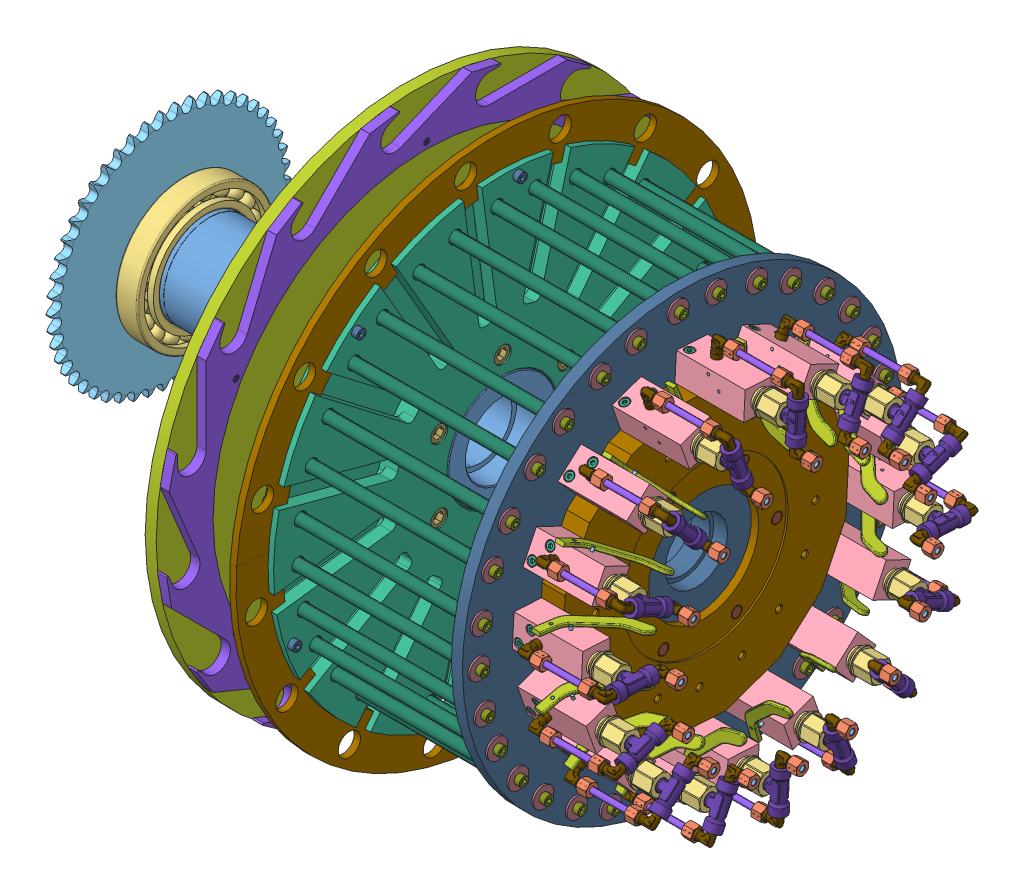
SolidWorks assembly assieme parte rotante, configuration Default. Lengths in mm. (continued)
Components (placement in the parent): (continued)
- AssiemeValvola-7: AssiemeValvola [Default] at (515.3257 -134.8578 488.6421) x (0 0.901303 -0.433189) z (0 -0.433189 -0.901303) size (90.26 138.63 38)
  - RaccordoT-1: RaccordoT [Default] at origin size (43 29.75 16.5)
  - Raccordo a L-1: Raccordo a L [Default] at (-30 0 0) x (0 -1 0) z (0 0 -1) size (28.34 25.51 14.01)
    - 1809_06_10_01-1: 1809_06_10_01 [Default] at origin size (22.49 23 10)
    - 1809_06_10_02-1: 1809_06_10_02 [Default] at origin size (6.5 8.5 8.5)
    - 1809_06_10_03-1: 1809_06_10_03 [Default] at origin size (11.02 15.01 14.01)
  - Raccordo a L-2: Raccordo a L [Default] at (30 0 0) x (0 1 0) z (0 0 -1) size (28.34 25.51 14.01)
    - 1809_06_10_01-1: 1809_06_10_01 [Default] at origin size (22.49 23 10)
    - 1809_06_10_02-1: 1809_06_10_02 [Default] at origin size (6.5 8.5 8.5)
    - 1809_06_10_03-1: 1809_06_10_03 [Default] at origin size (11.02 15.01 14.01)
  - TappoChiusura-1: TappoChiusura [Default] at (0 -32 0) x (0 -1 0) z (0 0 1) size (38.28 26.74 26.74)
  - CorpoValvola-1: CorpoValvola [Default] at (-15 -115.2824 0) size (30 75 34)
  - Raccordo a L-3: Raccordo a L [Default] at (-30 -88.2824 0) x (0 1 0) z (0 0 1) size (28.34 25.51 14.01)
    - 1809_06_10_01-1: 1809_06_10_01 [Default] at origin size (22.49 23 10)
    - 1809_06_10_02-1: 1809_06_10_02 [Default] at origin size (6.5 8.5 8.5)
    - 1809_06_10_03-1: 1809_06_10_03 [Default] at origin size (11.02 15.01 14.01)
  - Spina_3x38-1: Spina_3x38 [Default] at (0 -68.2824 -21) x (-1 0 0) z (0 0 1) size (3 3 38)
  - Spina_3x38-2: Spina_3x38 [Default] at (-10 -80.2824 -21) x (0.996193 0.087174 0) z (0 0 1) size (3 3 38)
  - M5 40mm-3: M5 40mm [ISO 4762 M5 x 40 - 40N] at (-14.6 -108.7824 9) size (45 8.5 8.5)
  - M5 40mm-2: M5 40mm [ISO 4762 M5 x 40 - 40N] at (-14.6 -96.7824 -9) size (45 8.5 8.5)
  - LevaValvola-1: LevaValvola [Default] at (-24.507 -86.571 -17) x (0.996193 0.087174 0) z (0 0 1) size (77.55 60.2 4)
  - Tubo-1: Tubo [Default] at (-30 -15.9665 0) x (1 0 0) z (0 -1 0) size (6 6 56.4)
- AssiemeValvola-8: AssiemeValvola [Default] at (515.3257 -95.0129 541.6718) x (0 0.666921 -0.745128) z (0 -0.745128 -0.666921) size (90.26 138.63 38)
  - RaccordoT-1: RaccordoT [Default] at origin size (43 29.75 16.5)
  - Raccordo a L-1: Raccordo a L [Default] at (-30 0 0) x (0 -1 0) z (0 0 -1) size (28.34 25.51 14.01)
    - 1809_06_10_01-1: 1809_06_10_01 [Default] at origin size (22.49 23 10)
    - 1809_06_10_02-1: 1809_06_10_02 [Default] at origin size (6.5 8.5 8.5)
    - 1809_06_10_03-1: 1809_06_10_03 [Default] at origin size (11.02 15.01 14.01)
  - Raccordo a L-2: Raccordo a L [Default] at (30 0 0) x (0 1 0) z (0 0 -1) size (28.34 25.51 14.01)
    - 1809_06_10_01-1: 1809_06_10_01 [Default] at origin size (22.49 23 10)
    - 1809_06_10_02-1: 1809_06_10_02 [Default] at origin size (6.5 8.5 8.5)
    - 1809_06_10_03-1: 1809_06_10_03 [Default] at origin size (11.02 15.01 14.01)
  - TappoChiusura-1: TappoChiusura [Default] at (0 -32 0) x (0 -1 0) z (0 0 1) size (38.28 26.74 26.74)
  - CorpoValvola-1: CorpoValvola [Default] at (-15 -115.2824 0) size (30 75 34)
  - Raccordo a L-3: Raccordo a L [Default] at (-30 -88.2824 0) x (0 1 0) z (0 0 1) size (28.34 25.51 14.01)
    - 1809_06_10_01-1: 1809_06_10_01 [Default] at origin size (22.49 23 10)
    - 1809_06_10_02-1: 1809_06_10_02 [Default] at origin size (6.5 8.5 8.5)
    - 1809_06_10_03-1: 1809_06_10_03 [Default] at origin size (11.02 15.01 14.01)
  - Spina_3x38-1: Spina_3x38 [Default] at (0 -68.2824 -21) x (-1 0 0) z (0 0 1) size (3 3 38)
  - Spina_3x38-2: Spina_3x38 [Default] at (-10 -80.2824 -21) x (0.996193 0.087174 0) z (0 0 1) size (3 3 38)
  - M5 40mm-3: M5 40mm [ISO 4762 M5 x 40 - 40N] at (-14.6 -108.7824 9) size (45 8.5 8.5)
  - M5 40mm-2: M5 40mm [ISO 4762 M5 x 40 - 40N] at (-14.6 -96.7824 -9) size (45 8.5 8.5)
  - LevaValvola-1: LevaValvola [Default] at (-24.507 -86.571 -17) x (0.996193 0.087174 0) z (0 0 1) size (77.55 60.2 4)
  - Tubo-1: Tubo [Default] at (-30 -15.9665 0) x (1 0 0) z (0 -1 0) size (6 6 56.4)
- AssiemeValvola-9: AssiemeValvola [Default] at (515.3257 -37.9074 575.4168) x (0 0.331007 -0.943628) z (0 -0.943628 -0.331007) size (90.26 138.63 38)
  - RaccordoT-1: RaccordoT [Default] at origin size (43 29.75 16.5)
  - Raccordo a L-1: Raccordo a L [Default] at (-30 0 0) x (0 -1 0) z (0 0 -1) size (28.34 25.51 14.01)
    - 1809_06_10_01-1: 1809_06_10_01 [Default] at origin size (22.49 23 10)
    - 1809_06_10_02-1: 1809_06_10_02 [Default] at origin size (6.5 8.5 8.5)
    - 1809_06_10_03-1: 1809_06_10_03 [Default] at origin size (11.02 15.01 14.01)
  - Raccordo a L-2: Raccordo a L [Default] at (30 0 0) x (0 1 0) z (0 0 -1) size (28.34 25.51 14.01)
    - 1809_06_10_01-1: 1809_06_10_01 [Default] at origin size (22.49 23 10)
    - 1809_06_10_02-1: 1809_06_10_02 [Default] at origin size (6.5 8.5 8.5)
    - 1809_06_10_03-1: 1809_06_10_03 [Default] at origin size (11.02 15.01 14.01)
  - TappoChiusura-1: TappoChiusura [Default] at (0 -32 0) x (0 -1 0) z (0 0 1) size (38.28 26.74 26.74)
  - CorpoValvola-1: CorpoValvola [Default] at (-15 -115.2824 0) size (30 75 34)
  - Raccordo a L-3: Raccordo a L [Default] at (-30 -88.2824 0) x (0 1 0) z (0 0 1) size (28.34 25.51 14.01)
    - 1809_06_10_01-1: 1809_06_10_01 [Default] at origin size (22.49 23 10)
    - 1809_06_10_02-1: 1809_06_10_02 [Default] at origin size (6.5 8.5 8.5)
    - 1809_06_10_03-1: 1809_06_10_03 [Default] at origin size (11.02 15.01 14.01)
  - Spina_3x38-1: Spina_3x38 [Default] at (0 -68.2824 -21) x (-1 0 0) z (0 0 1) size (3 3 38)
  - Spina_3x38-2: Spina_3x38 [Default] at (-10 -80.2824 -21) x (0.996193 0.087174 0) z (0 0 1) size (3 3 38)
  - M5 40mm-3: M5 40mm [ISO 4762 M5 x 40 - 40N] at (-14.6 -108.7824 9) size (45 8.5 8.5)
  - M5 40mm-2: M5 40mm [ISO 4762 M5 x 40 - 40N] at (-14.6 -96.7824 -9) size (45 8.5 8.5)
  - LevaValvola-1: LevaValvola [Default] at (-24.507 -86.571 -17) x (0.996193 0.087174 0) z (0 0 1) size (77.55 60.2 4)
  - Tubo-1: Tubo [Default] at (-30 -15.9665 0) x (1 0 0) z (0 -1 0) size (6 6 56.4)
- AssiemeValvola-10: AssiemeValvola [Default] at (515.3257 27.7648 584.7399) x (0 -0.055301 -0.99847) z (0 -0.99847 0.055301) size (90.26 138.63 38)
  - RaccordoT-1: RaccordoT [Default] at origin size (43 29.75 16.5)
  - Raccordo a L-1: Raccordo a L [Default] at (-30 0 0) x (0 -1 0) z (0 0 -1) size (28.34 25.51 14.01)
    - 1809_06_10_01-1: 1809_06_10_01 [Default] at origin size (22.49 23 10)
    - 1809_06_10_02-1: 1809_06_10_02 [Default] at origin size (6.5 8.5 8.5)
    - 1809_06_10_03-1: 1809_06_10_03 [Default] at origin size (11.02 15.01 14.01)
  - Raccordo a L-2: Raccordo a L [Default] at (30 0 0) x (0 1 0) z (0 0 -1) size (28.34 25.51 14.01)
    - 1809_06_10_01-1: 1809_06_10_01 [Default] at origin size (22.49 23 10)
    - 1809_06_10_02-1: 1809_06_10_02 [Default] at origin size (6.5 8.5 8.5)
    - 1809_06_10_03-1: 1809_06_10_03 [Default] at origin size (11.02 15.01 14.01)
  - TappoChiusura-1: TappoChiusura [Default] at (0 -32 0) x (0 -1 0) z (0 0 1) size (38.28 26.74 26.74)
  - CorpoValvola-1: CorpoValvola [Default] at (-15 -115.2824 0) size (30 75 34)
  - Raccordo a L-3: Raccordo a L [Default] at (-30 -88.2824 0) x (0 1 0) z (0 0 1) size (28.34 25.51 14.01)
    - 1809_06_10_01-1: 1809_06_10_01 [Default] at origin size (22.49 23 10)
    - 1809_06_10_02-1: 1809_06_10_02 [Default] at origin size (6.5 8.5 8.5)
    - 1809_06_10_03-1: 1809_06_10_03 [Default] at origin size (11.02 15.01 14.01)
  - Spina_3x38-1: Spina_3x38 [Default] at (0 -68.2824 -21) x (-1 0 0) z (0 0 1) size (3 3 38)
  - Spina_3x38-2: Spina_3x38 [Default] at (-10 -80.2824 -21) x (0.996193 0.087174 0) z (0 0 1) size (3 3 38)
  - M5 40mm-3: M5 40mm [ISO 4762 M5 x 40 - 40N] at (-14.6 -108.7824 9) size (45 8.5 8.5)
  - M5 40mm-2: M5 40mm [ISO 4762 M5 x 40 - 40N] at (-14.6 -96.7824 -9) size (45 8.5 8.5)
  - LevaValvola-1: LevaValvola [Default] at (-24.507 -86.571 -17) x (0.996193 0.087174 0) z (0 0 1) size (77.55 60.2 4)
  - Tubo-1: Tubo [Default] at (-30 -15.9665 0) x (1 0 0) z (0 -1 0) size (6 6 56.4)
- AssiemeValvola-11: AssiemeValvola [Default] at (515.3257 92.0058 568.2215) x (0 -0.433189 -0.901303) z (0 -0.901303 0.433189) size (90.26 138.63 38)
  - RaccordoT-1: RaccordoT [Default] at origin size (43 29.75 16.5)
  - Raccordo a L-1: Raccordo a L [Default] at (-30 0 0) x (0 -1 0) z (0 0 -1) size (28.34 25.51 14.01)
    - 1809_06_10_01-1: 1809_06_10_01 [Default] at origin size (22.49 23 10)
    - 1809_06_10_02-1: 1809_06_10_02 [Default] at origin size (6.5 8.5 8.5)
    - 1809_06_10_03-1: 1809_06_10_03 [Default] at origin size (11.02 15.01 14.01)
  - Raccordo a L-2: Raccordo a L [Default] at (30 0 0) x (0 1 0) z (0 0 -1) size (28.34 25.51 14.01)
    - 1809_06_10_01-1: 1809_06_10_01 [Default] at origin size (22.49 23 10)
    - 1809_06_10_02-1: 1809_06_10_02 [Default] at origin size (6.5 8.5 8.5)
    - 1809_06_10_03-1: 1809_06_10_03 [Default] at origin size (11.02 15.01 14.01)
  - TappoChiusura-1: TappoChiusura [Default] at (0 -32 0) x (0 -1 0) z (0 0 1) size (38.28 26.74 26.74)
  - CorpoValvola-1: CorpoValvola [Default] at (-15 -115.2824 0) size (30 75 34)
  - Raccordo a L-3: Raccordo a L [Default] at (-30 -88.2824 0) x (0 1 0) z (0 0 1) size (28.34 25.51 14.01)
    - 1809_06_10_01-1: 1809_06_10_01 [Default] at origin size (22.49 23 10)
    - 1809_06_10_02-1: 1809_06_10_02 [Default] at origin size (6.5 8.5 8.5)
    - 1809_06_10_03-1: 1809_06_10_03 [Default] at origin size (11.02 15.01 14.01)
  - Spina_3x38-1: Spina_3x38 [Default] at (0 -68.2824 -21) x (-1 0 0) z (0 0 1) size (3 3 38)
  - Spina_3x38-2: Spina_3x38 [Default] at (-10 -80.2824 -21) x (0.996193 0.087174 0) z (0 0 1) size (3 3 38)
  - M5 40mm-3: M5 40mm [ISO 4762 M5 x 40 - 40N] at (-14.6 -108.7824 9) size (45 8.5 8.5)
  - M5 40mm-2: M5 40mm [ISO 4762 M5 x 40 - 40N] at (-14.6 -96.7824 -9) size (45 8.5 8.5)
  - LevaValvola-1: LevaValvola [Default] at (-24.507 -86.571 -17) x (0.996193 0.087174 0) z (0 0 1) size (77.55 60.2 4)
  - Tubo-1: Tubo [Default] at (-30 -15.9665 0) x (1 0 0) z (0 -1 0) size (6 6 56.4)
- AssiemeValvola-12: AssiemeValvola [Default] at (515.3257 145.0355 528.3766) x (0 -0.745128 -0.666921) z (0 -0.666921 0.745128) size (90.26 138.63 38)
  - RaccordoT-1: RaccordoT [Default] at origin size (43 29.75 16.5)
  - Raccordo a L-1: Raccordo a L [Default] at (-30 0 0) x (0 -1 0) z (0 0 -1) size (28.34 25.51 14.01)
    - 1809_06_10_01-1: 1809_06_10_01 [Default] at origin size (22.49 23 10)
    - 1809_06_10_02-1: 1809_06_10_02 [Default] at origin size (6.5 8.5 8.5)
    - 1809_06_10_03-1: 1809_06_10_03 [Default] at origin size (11.02 15.01 14.01)
  - Raccordo a L-2: Raccordo a L [Default] at (30 0 0) x (0 1 0) z (0 0 -1) size (28.34 25.51 14.01)
    - 1809_06_10_01-1: 1809_06_10_01 [Default] at origin size (22.49 23 10)
    - 1809_06_10_02-1: 1809_06_10_02 [Default] at origin size (6.5 8.5 8.5)
    - 1809_06_10_03-1: 1809_06_10_03 [Default] at origin size (11.02 15.01 14.01)
  - TappoChiusura-1: TappoChiusura [Default] at (0 -32 0) x (0 -1 0) z (0 0 1) size (38.28 26.74 26.74)
  - CorpoValvola-1: CorpoValvola [Default] at (-15 -115.2824 0) size (30 75 34)
  - Raccordo a L-3: Raccordo a L [Default] at (-30 -88.2824 0) x (0 1 0) z (0 0 1) size (28.34 25.51 14.01)
    - 1809_06_10_01-1: 1809_06_10_01 [Default] at origin size (22.49 23 10)
    - 1809_06_10_02-1: 1809_06_10_02 [Default] at origin size (6.5 8.5 8.5)
    - 1809_06_10_03-1: 1809_06_10_03 [Default] at origin size (11.02 15.01 14.01)
  - Spina_3x38-1: Spina_3x38 [Default] at (0 -68.2824 -21) x (-1 0 0) z (0 0 1) size (3 3 38)
  - Spina_3x38-2: Spina_3x38 [Default] at (-10 -80.2824 -21) x (0.996193 0.087174 0) z (0 0 1) size (3 3 38)
  - M5 40mm-3: M5 40mm [ISO 4762 M5 x 40 - 40N] at (-14.6 -108.7824 9) size (45 8.5 8.5)
  - M5 40mm-2: M5 40mm [ISO 4762 M5 x 40 - 40N] at (-14.6 -96.7824 -9) size (45 8.5 8.5)
  - LevaValvola-1: LevaValvola [Default] at (-24.507 -86.571 -17) x (0.996193 0.087174 0) z (0 0 1) size (77.55 60.2 4)
  - Tubo-1: Tubo [Default] at (-30 -15.9665 0) x (1 0 0) z (0 -1 0) size (6 6 56.4)
- AssiemeValvola-13: AssiemeValvola [Default] at (515.3257 178.7805 471.2711) x (0 -0.943628 -0.331007) z (0 -0.331007 0.943628) size (90.26 138.63 38)
  - RaccordoT-1: RaccordoT [Default] at origin size (43 29.75 16.5)
  - Raccordo a L-1: Raccordo a L [Default] at (-30 0 0) x (0 -1 0) z (0 0 -1) size (28.34 25.51 14.01)
    - 1809_06_10_01-1: 1809_06_10_01 [Default] at origin size (22.49 23 10)
    - 1809_06_10_02-1: 1809_06_10_02 [Default] at origin size (6.5 8.5 8.5)
    - 1809_06_10_03-1: 1809_06_10_03 [Default] at origin size (11.02 15.01 14.01)
  - Raccordo a L-2: Raccordo a L [Default] at (30 0 0) x (0 1 0) z (0 0 -1) size (28.34 25.51 14.01)
    - 1809_06_10_01-1: 1809_06_10_01 [Default] at origin size (22.49 23 10)
    - 1809_06_10_02-1: 1809_06_10_02 [Default] at origin size (6.5 8.5 8.5)
    - 1809_06_10_03-1: 1809_06_10_03 [Default] at origin size (11.02 15.01 14.01)
  - TappoChiusura-1: TappoChiusura [Default] at (0 -32 0) x (0 -1 0) z (0 0 1) size (38.28 26.74 26.74)
  - CorpoValvola-1: CorpoValvola [Default] at (-15 -115.2824 0) size (30 75 34)
  - Raccordo a L-3: Raccordo a L [Default] at (-30 -88.2824 0) x (0 1 0) z (0 0 1) size (28.34 25.51 14.01)
    - 1809_06_10_01-1: 1809_06_10_01 [Default] at origin size (22.49 23 10)
    - 1809_06_10_02-1: 1809_06_10_02 [Default] at origin size (6.5 8.5 8.5)
    - 1809_06_10_03-1: 1809_06_10_03 [Default] at origin size (11.02 15.01 14.01)
  - Spina_3x38-1: Spina_3x38 [Default] at (0 -68.2824 -21) x (-1 0 0) z (0 0 1) size (3 3 38)
  - Spina_3x38-2: Spina_3x38 [Default] at (-10 -80.2824 -21) x (0.996193 0.087174 0) z (0 0 1) size (3 3 38)
  - M5 40mm-3: M5 40mm [ISO 4762 M5 x 40 - 40N] at (-14.6 -108.7824 9) size (45 8.5 8.5)
  - M5 40mm-2: M5 40mm [ISO 4762 M5 x 40 - 40N] at (-14.6 -96.7824 -9) size (45 8.5 8.5)
  - LevaValvola-1: LevaValvola [Default] at (-24.507 -86.571 -17) x (0.996193 0.087174 0) z (0 0 1) size (77.55 60.2 4)
  - Tubo-1: Tubo [Default] at (-30 -15.9665 0) x (1 0 0) z (0 -1 0) size (6 6 56.4)
- AssiemeValvola-14: AssiemeValvola [Default] at (515.3257 188.1036 405.5989) x (0 -0.99847 0.055301) z (0 0.055301 0.99847) size (90.26 138.63 38)
  - RaccordoT-1: RaccordoT [Default] at origin size (43 29.75 16.5)
  - Raccordo a L-1: Raccordo a L [Default] at (-30 0 0) x (0 -1 0) z (0 0 -1) size (28.34 25.51 14.01)
    - 1809_06_10_01-1: 1809_06_10_01 [Default] at origin size (22.49 23 10)
    - 1809_06_10_02-1: 1809_06_10_02 [Default] at origin size (6.5 8.5 8.5)
    - 1809_06_10_03-1: 1809_06_10_03 [Default] at origin size (11.02 15.01 14.01)
  - Raccordo a L-2: Raccordo a L [Default] at (30 0 0) x (0 1 0) z (0 0 -1) size (28.34 25.51 14.01)
    - 1809_06_10_01-1: 1809_06_10_01 [Default] at origin size (22.49 23 10)
    - 1809_06_10_02-1: 1809_06_10_02 [Default] at origin size (6.5 8.5 8.5)
    - 1809_06_10_03-1: 1809_06_10_03 [Default] at origin size (11.02 15.01 14.01)
  - TappoChiusura-1: TappoChiusura [Default] at (0 -32 0) x (0 -1 0) z (0 0 1) size (38.28 26.74 26.74)
  - CorpoValvola-1: CorpoValvola [Default] at (-15 -115.2824 0) size (30 75 34)
  - Raccordo a L-3: Raccordo a L [Default] at (-30 -88.2824 0) x (0 1 0) z (0 0 1) size (28.34 25.51 14.01)
    - 1809_06_10_01-1: 1809_06_10_01 [Default] at origin size (22.49 23 10)
    - 1809_06_10_02-1: 1809_06_10_02 [Default] at origin size (6.5 8.5 8.5)
    - 1809_06_10_03-1: 1809_06_10_03 [Default] at origin size (11.02 15.01 14.01)
  - Spina_3x38-1: Spina_3x38 [Default] at (0 -68.2824 -21) x (-1 0 0) z (0 0 1) size (3 3 38)
  - Spina_3x38-2: Spina_3x38 [Default] at (-10 -80.2824 -21) x (0.996193 0.087174 0) z (0 0 1) size (3 3 38)
  - M5 40mm-3: M5 40mm [ISO 4762 M5 x 40 - 40N] at (-14.6 -108.7824 9) size (45 8.5 8.5)
  - M5 40mm-2: M5 40mm [ISO 4762 M5 x 40 - 40N] at (-14.6 -96.7824 -9) size (45 8.5 8.5)
  - LevaValvola-1: LevaValvola [Default] at (-24.507 -86.571 -17) x (0.996193 0.087174 0) z (0 0 1) size (77.55 60.2 4)
  - Tubo-1: Tubo [Default] at (-30 -15.9665 0) x (1 0 0) z (0 -1 0) size (6 6 56.4)
- AssiemeValvola-15: AssiemeValvola [Default] at (515.3257 171.5852 341.3579) x (0 -0.901303 0.433189) z (0 0.433189 0.901303) size (90.26 138.63 38)
  - RaccordoT-1: RaccordoT [Default] at origin size (43 29.75 16.5)
  - Raccordo a L-1: Raccordo a L [Default] at (-30 0 0) x (0 -1 0) z (0 0 -1) size (28.34 25.51 14.01)
    - 1809_06_10_01-1: 1809_06_10_01 [Default] at origin size (22.49 23 10)
    - 1809_06_10_02-1: 1809_06_10_02 [Default] at origin size (6.5 8.5 8.5)
    - 1809_06_10_03-1: 1809_06_10_03 [Default] at origin size (11.02 15.01 14.01)
  - Raccordo a L-2: Raccordo a L [Default] at (30 0 0) x (0 1 0) z (0 0 -1) size (28.34 25.51 14.01)
    - 1809_06_10_01-1: 1809_06_10_01 [Default] at origin size (22.49 23 10)
    - 1809_06_10_02-1: 1809_06_10_02 [Default] at origin size (6.5 8.5 8.5)
    - 1809_06_10_03-1: 1809_06_10_03 [Default] at origin size (11.02 15.01 14.01)
  - TappoChiusura-1: TappoChiusura [Default] at (0 -32 0) x (0 -1 0) z (0 0 1) size (38.28 26.74 26.74)
  - CorpoValvola-1: CorpoValvola [Default] at (-15 -115.2824 0) size (30 75 34)
  - Raccordo a L-3: Raccordo a L [Default] at (-30 -88.2824 0) x (0 1 0) z (0 0 1) size (28.34 25.51 14.01)
    - 1809_06_10_01-1: 1809_06_10_01 [Default] at origin size (22.49 23 10)
    - 1809_06_10_02-1: 1809_06_10_02 [Default] at origin size (6.5 8.5 8.5)
    - 1809_06_10_03-1: 1809_06_10_03 [Default] at origin size (11.02 15.01 14.01)
  - Spina_3x38-1: Spina_3x38 [Default] at (0 -68.2824 -21) x (-1 0 0) z (0 0 1) size (3 3 38)
  - Spina_3x38-2: Spina_3x38 [Default] at (-10 -80.2824 -21) x (0.996193 0.087174 0) z (0 0 1) size (3 3 38)
  - M5 40mm-3: M5 40mm [ISO 4762 M5 x 40 - 40N] at (-14.6 -108.7824 9) size (45 8.5 8.5)
  - M5 40mm-2: M5 40mm [ISO 4762 M5 x 40 - 40N] at (-14.6 -96.7824 -9) size (45 8.5 8.5)
  - LevaValvola-1: LevaValvola [Default] at (-24.507 -86.571 -17) x (0.996193 0.087174 0) z (0 0 1) size (77.55 60.2 4)
  - Tubo-1: Tubo [Default] at (-30 -15.9665 0) x (1 0 0) z (0 -1 0) size (6 6 56.4)
- AssiemeValvola-16: AssiemeValvola [Default] at (515.3257 131.7403 288.3282) x (0 -0.666921 0.745128) z (0 0.745128 0.666921) size (90.26 138.63 38)
  - RaccordoT-1: RaccordoT [Default] at origin size (43 29.75 16.5)
  - Raccordo a L-1: Raccordo a L [Default] at (-30 0 0) x (0 -1 0) z (0 0 -1) size (28.34 25.51 14.01)
    - 1809_06_10_01-1: 1809_06_10_01 [Default] at origin size (22.49 23 10)
    - 1809_06_10_02-1: 1809_06_10_02 [Default] at origin size (6.5 8.5 8.5)
    - 1809_06_10_03-1: 1809_06_10_03 [Default] at origin size (11.02 15.01 14.01)
  - Raccordo a L-2: Raccordo a L [Default] at (30 0 0) x (0 1 0) z (0 0 -1) size (28.34 25.51 14.01)
    - 1809_06_10_01-1: 1809_06_10_01 [Default] at origin size (22.49 23 10)
    - 1809_06_10_02-1: 1809_06_10_02 [Default] at origin size (6.5 8.5 8.5)
    - 1809_06_10_03-1: 1809_06_10_03 [Default] at origin size (11.02 15.01 14.01)
  - TappoChiusura-1: TappoChiusura [Default] at (0 -32 0) x (0 -1 0) z (0 0 1) size (38.28 26.74 26.74)
  - CorpoValvola-1: CorpoValvola [Default] at (-15 -115.2824 0) size (30 75 34)
  - Raccordo a L-3: Raccordo a L [Default] at (-30 -88.2824 0) x (0 1 0) z (0 0 1) size (28.34 25.51 14.01)
    - 1809_06_10_01-1: 1809_06_10_01 [Default] at origin size (22.49 23 10)
    - 1809_06_10_02-1: 1809_06_10_02 [Default] at origin size (6.5 8.5 8.5)
    - 1809_06_10_03-1: 1809_06_10_03 [Default] at origin size (11.02 15.01 14.01)
  - Spina_3x38-1: Spina_3x38 [Default] at (0 -68.2824 -21) x (-1 0 0) z (0 0 1) size (3 3 38)
  - Spina_3x38-2: Spina_3x38 [Default] at (-10 -80.2824 -21) x (0.996193 0.087174 0) z (0 0 1) size (3 3 38)
  - M5 40mm-3: M5 40mm [ISO 4762 M5 x 40 - 40N] at (-14.6 -108.7824 9) size (45 8.5 8.5)
  - M5 40mm-2: M5 40mm [ISO 4762 M5 x 40 - 40N] at (-14.6 -96.7824 -9) size (45 8.5 8.5)
  - LevaValvola-1: LevaValvola [Default] at (-24.507 -86.571 -17) x (0.996193 0.087174 0) z (0 0 1) size (77.55 60.2 4)
  - Tubo-1: Tubo [Default] at (-30 -15.9665 0) x (1 0 0) z (0 -1 0) size (6 6 56.4)
- Disco alimentazione guarnizione fi24.4-1: Disco alimentazione guarnizione fi24.4 [Default] at (198.0433 18.3637 415) x (0 0.065403 0.997859) z (-1 0 0) size (570 285 7.35)
- Disco alimentazione guarnizione fi24.4-2: Disco alimentazione guarnizione fi24.4 [Default] at (198.0433 18.3637 415) x (0 -0.065403 -0.997859) z (-1 0 0) size (570 285 7.35)
- m6 12mm-1: m6 12mm [ISO 4762 M6 x 12 - 12N] at (210.0433 200.6849 574.8914) x (-1 0 0) z (0 0.793353 -0.608761) size (18 10 10)
- m6 12mm-7: m6 12mm [ISO 4762 M6 x 12 - 12N] at (210.0433 260.3445 399.1397) x (-1 0 0) z (0 0.793353 -0.608761) size (18 10 10)
- m6 12mm-8: m6 12mm [ISO 4762 M6 x 12 - 12N] at (210.0433 96.3128 185.3694) x (-1 0 0) z (0 0.793353 -0.608761) size (18 10 10)
- m6 12mm-9: m6 12mm [ISO 4762 M6 x 12 - 12N] at (210.0433 -59.5854 644.6306) x (-1 0 0) z (0 -0.793353 -0.608761) size (18 10 10)
- m6 12mm-10: m6 12mm [ISO 4762 M6 x 12 - 12N] at (210.0433 -223.6171 430.8603) x (-1 0 0) z (0 -0.793353 -0.608761) size (18 10 10)
- m6 12mm-11: m6 12mm [ISO 4762 M6 x 12 - 12N] at (210.0433 -163.9575 255.1086) x (-1 0 0) z (0 0.793353 -0.608761) size (18 10 10)
Mates (geometry in assembly coordinates):
- Concentrico1: concentric anti-aligned: circle of albero rotazione piatti-1; circle of seger 100mm-1
- Coincidente1: coincident anti-aligned: plane of albero rotazione piatti-1 through (-143.4567 18.3637 415) normal (-1 0 0); plane of seger 100mm-1 through (-143.4567 18.3637 415) normal (1 0 0)
- Coincidente2: coincident aligned: plane of albero rotazione piatti-1 through (60.413 18.3637 415) normal (0 1 0); plane of seger 100mm-1 through (-146.4567 18.3637 415) normal (0 1 0)
- Concentrico21: concentric aligned: cylinder of albero rotazione piatti-1 through (60.413 18.3637 415) axis (1 0 0) radius 50; cylinder of SKF - 6020 - 20,DE,NC,20_68-1 through (-152.0942 18.3637 415) axis (1 0 0) radius 50
- Coincidente3: coincident anti-aligned: plane of seger 100mm-1 through (-143.4567 18.3637 415) normal (1 0 0); plane of SKF - 6020 - 20,DE,NC,20_68-1 through (-143.4567 -33.4256 439.9823) normal (-1 0 0)
- Concentrico3: concentric aligned: cylinder of albero rotazione piatti-1 through (60.413 18.3637 415) axis (1 0 0) radius 47.5; cylinder of calettatore d95-1 through (-193.8867 18.3637 415) axis (1 0 0) radius 47.5
- Coincidente7: coincident aligned: plane of albero rotazione piatti-1 through (60.413 18.3637 415) normal (0 1 0); plane of calettatore d95-1 through (-178.8867 18.3637 415) normal (0 1 0)
- Concentrico5: concentric aligned: cylinder of albero rotazione piatti-1 through (60.413 18.3637 415) axis (1 0 0) radius 49.75; cylinder of SKF - 6020 - 20,DE,NC,20_68-2 through (41.4058 18.3637 415) axis (1 0 0) radius 50
- Coincidente8: coincident anti-aligned: plane of albero rotazione piatti-1 through (74.0433 18.3637 415) normal (-1 0 0); plane of SKF - 6020 - 20,DE,NC,20_68-2 through (74.0433 -28.0673 437.2803) normal (1 0 0)
- Concentrico6: concentric aligned: cylinder of albero rotazione piatti-1 through (60.413 18.3637 415) axis (1 0 0) radius 60; cylinder of Disco supporto montaggio e Colonne-1 through (5.3377 18.3637 415) axis (1 0 0) radius 60
- Concentrico7: concentric aligned: cylinder of albero rotazione piatti-1 through (101.3656 98.3637 415) axis (1 0 0) radius 6.25; cylinder of Disco supporto montaggio e Colonne-1 through (204.0433 98.3637 415) axis (1 0 0) radius 9.25
- Coincidente9: coincident anti-aligned: plane of albero rotazione piatti-1 through (175.0433 18.3637 415) normal (1 0 0); plane of Disco supporto montaggio e Colonne-1 through (175.0433 18.3637 415) normal (-1 0 0)
- Concentrico8: concentric anti-aligned: cylinder of albero rotazione piatti-1 through (60.413 18.3637 415) axis (1 0 0) radius 60; cylinder of piatto rotante porta tappi-1 through (111.0433 18.3637 415) axis (-1 0 0) radius 60
- Concentrico9: concentric aligned: circle of albero rotazione piatti-1; circle of piatto rotante porta tappi-1
- Coincidente10: coincident anti-aligned: plane of albero rotazione piatti-1 through (119.0433 18.3637 415) normal (-1 0 0); plane of piatto rotante porta tappi-1 through (119.0433 18.3637 415) normal (1 0 0)
- Concentrico10: concentric aligned: cylinder of piatto rotante porta tappi-1 through (119.0433 18.3637 415) axis (-1 0 0) radius 233; cylinder of disco trasportatore tappi 31-1 through (121.0433 18.3637 415) axis (-1 0 0) radius 233
- Tangente2: tangent: cylinder of piatto rotante porta tappi-1 through (98.5243 -101.6363 622.8461) axis (1 0 0) radius 3.25; curve of disco trasportatore tappi 31-1
- Coincidente13: coincident anti-aligned: plane of piatto rotante porta tappi-1 through (111.0433 18.3637 415) normal (1 0 0); plane of disco trasportatore tappi 31-1 through (111.0433 18.3637 415) normal (-1 0 0)
- Concentrico11: concentric anti-aligned: cylinder of albero rotazione piatti-1 through (60.413 18.3637 415) axis (1 0 0) radius 40; cylinder of disco trascinato porta distributore vuoto-1 through (400.0433 18.3637 415) axis (-1 0 0) radius 30
- Concentrico12: concentric anti-aligned: cylinder of Disco supporto montaggio e Colonne-1 through (204.0433 -202.0247 450.2415) axis (1 0 0) radius 6; cylinder of disco trascinato porta distributore vuoto-1 through (417.0139 -202.0247 450.2415) axis (-1 0 0) radius 6
- Coincidente14: coincident anti-aligned: plane of Distributore Rotante-1 through (400.0433 18.3637 415) normal (-1 0 0); plane of disco trascinato porta distributore vuoto-1 through (400.0433 18.3637 415) normal (1 0 0)
- Concentrico13: concentric anti-aligned: circle of Distributore Rotante-1; circle of disco trascinato porta distributore vuoto-1
- Concentrico14: concentric anti-aligned: cylinder of Distributore Rotante-1 through (230.3377 18.3637 415) axis (1 0 0) radius 60; cylinder of disco trascinato porta distributore vuoto-1 through (415.0433 18.3637 415) axis (-1 0 0) radius 67.5
- Concentrico15: concentric anti-aligned: cylinder of disco trascinato porta distributore vuoto-1 through (388.0433 -53.0243 378.8925) axis (1 0 0) radius 6.25; cylinder of m12 35mm-1 through (344.2933 -53.0243 378.8925) axis (-1 0 0) radius 6
- Coincidente15: coincident anti-aligned: plane of disco trascinato porta distributore vuoto-1 through (388.0433 18.3637 415) normal (-1 0 0); plane of m12 35mm-1 through (388.0433 -45.2301 383.3925) normal (1 0 0)
- Parallelo1: parallel anti-aligned: plane of m12 35mm-1 through (382.0433 -47.9668 381.8125) normal (0 -1 0)
- Concentrico16: concentric aligned: cylinder of Disco supporto montaggio e Colonne-1 through (204.0433 -21.6363 345.718) axis (1 0 0) radius 9.25; cylinder of m12 90mm-3 through (234.7933 -21.6363 345.718) axis (1 0 0) radius 6
- Coincidente17: coincident anti-aligned: plane of Disco supporto montaggio e Colonne-1 through (191.0433 -27.049 342.593) normal (1 0 0); plane of m12 90mm-3 through (191.0433 -29.4305 341.218) normal (-1 0 0)
- Parallelo2: parallel aligned: plane of m12 35mm-1 through (382.0433 -47.9668 381.8125) normal (0 -1 0); plane of m12 90mm-3 through (197.0433 -16.5788 348.6379) normal (0 -1 0)
- Concentrico171: concentric anti-aligned: cylinder of piatto rotante porta tappi-1 through (98.5243 -101.6363 207.1539) axis (1 0 0) radius 3.25; cylinder of rondella m6 22mm-1 through (64.1183 -101.6363 207.1539) axis (-1 0 0) radius 3.3
- Coincidente191: coincident anti-aligned: plane of piatto rotante porta tappi-1 through (99.0433 18.3637 415) normal (-1 0 0); plane of rondella m6 22mm-1 through (99.0433 -101.6363 210.4539) normal (1 0 0)
- Parallelo3: parallel anti-aligned: plane of rondella m6 22mm-1 through (99.0433 -101.6363 207.1539) normal (0 -1 0)
- Concentrico181: concentric aligned: cylinder of rondella m6 22mm-1 through (64.1183 -101.6363 207.1539) axis (-1 0 0) radius 3.3; cylinder of M6 20mm-1 through (59.2933 -101.6363 207.1539) axis (-1 0 0) radius 5
- Coincidente211: coincident anti-aligned: plane of rondella m6 22mm-1 through (97.0433 -101.6363 218.1539) normal (-1 0 0); plane of M6 20mm-1 through (97.0433 -97.3062 204.6539) normal (1 0 0)
- Parallelo4: parallel aligned: plane of m12 35mm-1 through (382.0433 -47.9668 381.8125) normal (0 -0.5 -0.866025); plane of M6 20mm-1 through (94.0433 -101.6363 210.0892) normal (0 -0.5 -0.866025)
- Concentrico19: concentric anti-aligned: cylinder of Disco supporto montaggio e Colonne-1 through (204.0433 70.1437 197.9013) axis (1 0 0) radius 6; cylinder of asta scorrimento carello-1 through (400.0433 70.1437 197.9013) axis (-1 0 0) radius 6
- Concentrico201: concentric aligned: cylinder of asta scorrimento carello-1 through (175.0433 70.1437 197.9013) axis (-1 0 0) radius 3.2; cylinder of rondella m6 22mm-7 through (140.1183 70.1437 197.9013) axis (-1 0 0) radius 3.3
- Coincidente231: coincident anti-aligned: plane of asta scorrimento carello-1 through (175.0433 70.1437 197.9013) normal (-1 0 0); plane of rondella m6 22mm-7 through (175.0433 70.1437 201.2013) normal (1 0 0)
- Concentrico211: concentric aligned: cylinder of rondella m6 22mm-7 through (140.1183 70.1437 197.9013) axis (-1 0 0) radius 3.3; cylinder of M6 16mm-1 through (135.2933 70.1437 197.9013) axis (-1 0 0) radius 5
- Coincidente241: coincident anti-aligned: plane of rondella m6 22mm-7 through (173.0433 70.1437 208.9013) normal (-1 0 0); plane of M6 16mm-1 through (173.0433 75.1437 197.9013) normal (1 0 0)
- Parallelo5: parallel aligned: plane of asta scorrimento carello-1 through (287.5433 70.1437 197.9013) normal (0 0 -1); plane of M6 16mm-1 through (170.0433 68.6761 200.4433) normal (0 0 -1)
- Parallelo9: parallel anti-aligned: plane of rondella m6 22mm-7 through (175.0433 70.1437 197.9013) normal (0 0 1); plane of M6 16mm-1 through (170.0433 68.6761 200.4433) normal (0 0 -1)
- Coincidente30: coincident anti-aligned: plane of Disco supporto montaggio e Colonne-1 through (175.0433 18.3637 415) normal (-1 0 0); plane of rondella m6 22mm-7 through (175.0433 70.1437 201.2013) normal (1 0 0)
- Coincidente31: coincident anti-aligned: plane of disco trascinato porta distributore vuoto-1 through (400.0433 18.3637 415) normal (1 0 0); plane of rondella m6 22mm-8 through (400.0433 70.1437 201.2013) normal (-1 0 0)
- Coincidente32: coincident anti-aligned: plane of Distributore Rotante-1 through (400.0433 40.5763 258.5322) normal (0 0.331007 -0.943628); plane of AssiemeValvola-1/CorpoValvola-1 through (400.0433 85.7114 274.3647) normal (0 -0.331007 0.943628)
- Coincidente33: coincident anti-aligned: plane of disco trascinato porta distributore vuoto-1 through (400.0433 18.3637 415) normal (1 0 0); plane of AssiemeValvola-1/CorpoValvola-1 through (400.0433 95.6416 246.0559) normal (-1 0 0)
- Concentrico22: concentric anti-aligned: cylinder of Distributore Rotante-1 through (412.5433 55.4365 309.3136) axis (0 0.331007 -0.943628) radius 3; cylinder of AssiemeValvola-1/CorpoValvola-1 through (412.5433 69.6697 268.7376) axis (0 -0.331007 0.943628) radius 3
- Concentrico23: concentric anti-aligned: cylinder of Disco supporto montaggio e Colonne-1 through (198.0433 18.3637 415) axis (-1 0 0) radius 235; cylinder of Disco alimentazione guarnizione fi24.4-2 through (191.0433 18.3637 415) axis (1 0 0) radius 235
- Concentrico24: concentric anti-aligned: cylinder of Disco supporto montaggio e Colonne-1 through (198.0433 18.3637 415) axis (-1 0 0) radius 235; cylinder of Disco alimentazione guarnizione fi24.4-1 through (191.0433 18.3637 415) axis (1 0 0) radius 235
- Coincidente34: coincident anti-aligned: plane of Disco alimentazione guarnizione fi24.4-1 through (191.0433 33.7334 649.4968) normal (0 -0.997859 0.065403); plane of Disco alimentazione guarnizione fi24.4-2 through (191.0433 37.0036 699.3898) normal (0 0.997859 -0.065403)
- Coincidente35: coincident aligned: plane of Disco alimentazione guarnizione fi24.4-1 through (198.0433 18.3637 415) normal (1 0 0); plane of Disco alimentazione guarnizione fi24.4-2 through (198.0433 18.3637 415) normal (1 0 0)
- Concentrico25: concentric anti-aligned: cylinder of Disco supporto montaggio e Colonne-1 through (188.8509 -59.5854 644.6306) axis (1 0 0) radius 3.25; circle of Disco alimentazione guarnizione fi24.4-2
- Coincidente36: coincident anti-aligned: plane of Disco supporto montaggio e Colonne-1 through (198.0433 18.3637 415) normal (-1 0 0); plane of Disco alimentazione guarnizione fi24.4-2 through (198.0433 18.3637 415) normal (1 0 0)
- Concentrico26: concentric anti-aligned: cylinder of Disco supporto montaggio e Colonne-1 through (188.8509 200.6849 574.8914) axis (1 0 0) radius 3.25; cylinder of M6 16mm-65 through (198.0564 200.6849 574.8914) axis (-1 0 0) radius 3
- Concentrico271: concentric anti-aligned: cone of Disco supporto montaggio e Colonne-1 through (203.0433 200.6849 574.8914) axis (-1 0 0); cylinder of m6 12mm-1 through (241.7933 200.6849 574.8914) axis (1 0 0) radius 5
- Coincidente381: coincident anti-aligned: plane of Disco supporto montaggio e Colonne-1 through (204.0433 18.3637 415) normal (1 0 0); plane of m6 12mm-1 through (204.0433 203.7287 578.8581) normal (-1 0 0)
- Concentrico281: concentric anti-aligned: cone of Disco supporto montaggio e Colonne-1 through (203.0433 260.3445 399.1397) axis (-1 0 0); cylinder of m6 12mm-7 through (241.7933 260.3445 399.1397) axis (1 0 0) radius 5
- Coincidente401: coincident anti-aligned: plane of Disco supporto montaggio e Colonne-1 through (204.0433 18.3637 415) normal (1 0 0); plane of m6 12mm-7 through (204.0433 263.3883 403.1065) normal (-1 0 0)
- Parallelo11: parallel aligned: plane of m6 12mm-1 through (207.0433 198.898 572.5627) normal (0 0.92388 0.382683); plane of m6 12mm-7 through (207.0433 258.5576 396.8111) normal (0 0.92388 0.382683)
- Concentrico291: concentric anti-aligned: cone of Disco supporto montaggio e Colonne-1 through (203.0433 96.3128 185.3694) axis (-1 0 0); cylinder of m6 12mm-8 through (241.7933 96.3128 185.3694) axis (1 0 0) radius 5
- Coincidente421: coincident anti-aligned: plane of Disco supporto montaggio e Colonne-1 through (204.0433 18.3637 415) normal (1 0 0); plane of m6 12mm-8 through (204.0433 99.3566 189.3362) normal (-1 0 0)
- Coincidente44: coincident aligned: plane of m6 12mm-7 through (207.0433 259.2212 401.8516) normal (0 0.793353 -0.608761); plane of m6 12mm-8 through (207.0433 95.1895 188.0813) normal (0 0.793353 -0.608761)
- Concentrico301: concentric anti-aligned: cone of Disco supporto montaggio e Colonne-1 through (203.0433 -59.5854 644.6306) axis (-1 0 0); cylinder of m6 12mm-9 through (241.7933 -59.5854 644.6306) axis (1 0 0) radius 5
- Coincidente451: coincident anti-aligned: plane of Disco supporto montaggio e Colonne-1 through (204.0433 18.3637 415) normal (1 0 0); plane of m6 12mm-9 through (204.0433 -56.5416 640.6638) normal (-1 0 0)
- Concentrico311: concentric anti-aligned: cone of Disco supporto montaggio e Colonne-1 through (203.0433 -223.6171 430.8603) axis (-1 0 0); cylinder of m6 12mm-10 through (241.7933 -223.6171 430.8603) axis (1 0 0) radius 5
- Coincidente461: coincident anti-aligned: plane of Disco supporto montaggio e Colonne-1 through (204.0433 18.3637 415) normal (1 0 0); plane of m6 12mm-10 through (204.0433 -220.5733 426.8935) normal (-1 0 0)
- Concentrico321: concentric anti-aligned: cone of Disco supporto montaggio e Colonne-1 through (203.0433 -163.9575 255.1086) axis (-1 0 0); cylinder of m6 12mm-11 through (241.7933 -163.9575 255.1086) axis (1 0 0) radius 5
- Coincidente471: coincident anti-aligned: plane of Disco supporto montaggio e Colonne-1 through (204.0433 18.3637 415) normal (1 0 0); plane of m6 12mm-11 through (204.0433 -160.9136 259.0754) normal (-1 0 0)
- Parallelo13: parallel aligned: plane of m6 12mm-9 through (207.0433 -62.4955 644.2474) normal (0 0.92388 -0.382683); plane of m6 12mm-10 through (207.0433 -226.5272 430.4771) normal (0 0.92388 -0.382683)
- Parallelo14: parallel aligned: plane of Disco supporto montaggio e Colonne-1 through (191.0433 26.2972 408.9124) normal (0 -0.793353 0.608761); plane of m6 12mm-11 through (207.0433 -162.8342 252.3968) normal (0 -0.793353 0.608761)
- Parallelo15: parallel aligned: plane of Disco supporto montaggio e Colonne-1 through (191.0433 19.669 405.0856) normal (0 -0.130526 0.991445); plane of m6 12mm-10 through (207.0433 -221.8302 428.5316) normal (0 -0.130526 0.991445)
- Concentrico322: concentric anti-aligned: cylinder of albero rotazione piatti-1 through (60.413 18.3637 415) axis (1 0 0) radius 47.5; cylinder of Chain wheel ISO - 50Z 10A-1-1 through (-139.8862 18.3637 415) axis (-1 0 0) radius 47.5
- Coincidente472: coincident anti-aligned: plane of albero rotazione piatti-1 through (-155.9567 18.3637 415) normal (-1 0 0); plane of Chain wheel ISO - 50Z 10A-1-1 through (-155.9567 18.3637 415) normal (1 0 0)
- Concentrico323: concentric: cylinder of calettatore d95-1 through (-190.8867 18.3637 415) axis (1 0 0) radius 67.5; cylinder of Chain wheel ISO - 50Z 10A-1-1 through (-164.8867 18.3637 415) axis (-1 0 0) radius 67.5
- Coincidente473: coincident: plane of calettatore d95-1 through (-164.8867 84.9137 415) normal (1 0 0); plane of Chain wheel ISO - 50Z 10A-1-1 through (-164.8867 18.3637 415) normal (-1 0 0)
- Parallelo16: parallel aligned: plane of Chain wheel ISO - 50Z 10A-1-1 through (-164.8867 18.3637 415) normal (0 1 0)
- Parallelo17: parallel aligned: plane of calettatore d95-1 through (-178.8867 18.3637 415) normal (0 1 0)
